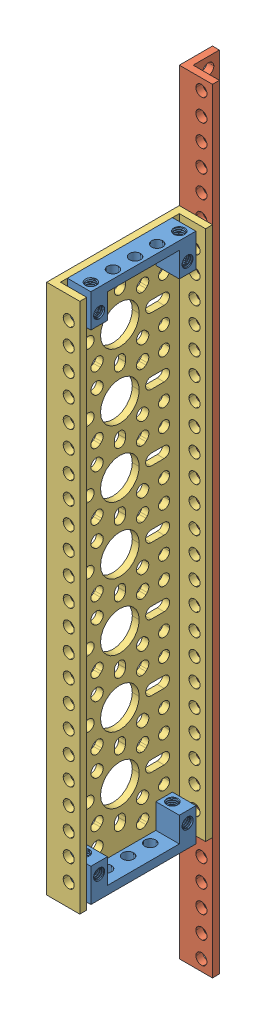
SolidWorks assembly Elevator Chassis Bridge, configuration Default. Lengths in mm.
Overall size (12 280 60).
4 component instances, 3 part files, 6 mates.
Components (placement in the parent):
- Dual Block.step-1: Dual Block.step [Default] at (-105.3931 154.1344 373.8846) size (8.51 12.01 38)
- Dual Block.step-2: Dual Block.step [Default] at (-139.8931 -13.8656 373.8846) x (-1 0 0) z (0 0 1) size (8.51 12.01 38)
- 35 Hole L Beam.step-1: 35 Hole L Beam.step [Default] at (-129.3931 -69.8656 349.8846) size (12 280 12)
- Thin 7-2: Thin 7 [Default] at (-105.3931 -25.8656 395.3846) size (12 192 48)
Mates (geometry in assembly coordinates):
- Coincident31: coincident: circle of Dual Block.step-1; circle of Thin 7-2
- Coincident37: coincident: circle of Dual Block.step-2; circle of Thin 7-2
- Concentric20: concentric: circle of Dual Block.step-2; circle of Thin 7-2
- Concentric21: concentric: circle of Dual Block.step-1; circle of Thin 7-2
- Coincident40: coincident: circle of 35 Hole L Beam.step-1; circle of Thin 7-2
- Concentric22: concentric: cylinder of 35 Hole L Beam.step-1 through (-121.3931 -17.8656 337.8846) axis (0 0 1) radius 2; cylinder of Thin 7-2 through (-121.3931 -17.8656 349.8846) axis (0 0 1) radius 2
